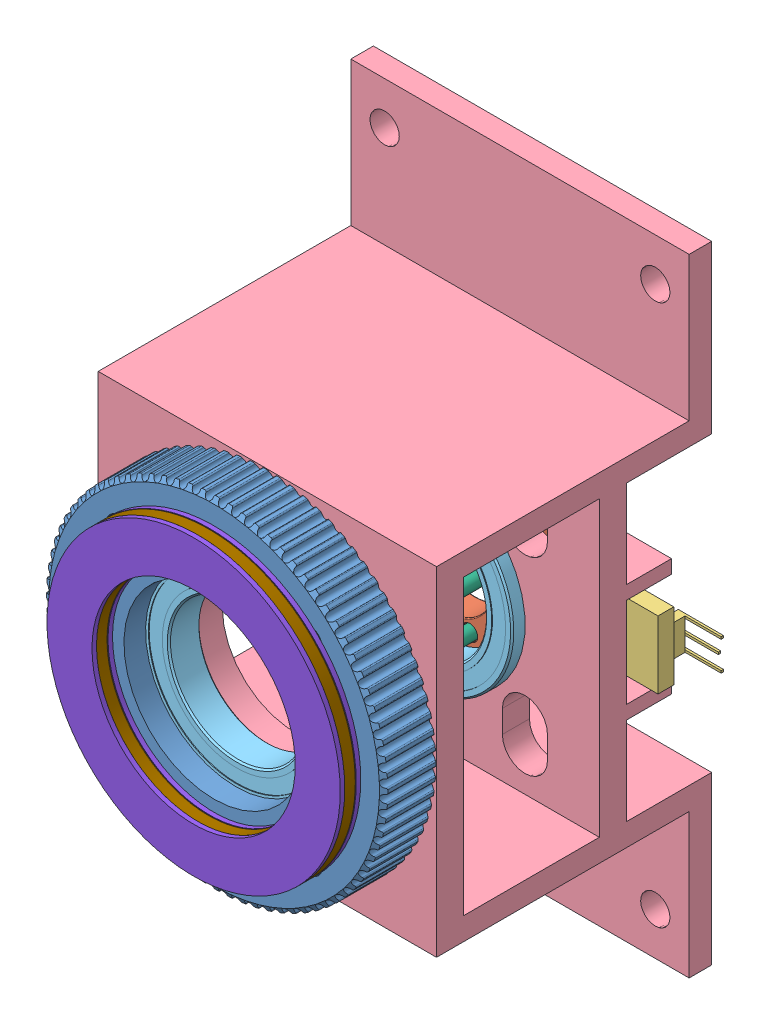
SolidWorks assembly Assem4, configuration Default. Lengths in mm.
Overall size (90.97 138.93 77.35).
21 component instances, 9 part files, 41 mates.
Components (placement in the parent):
- pulleyHTD3m80Tbase-1: pulleyHTD3m80Tbase [Default] at (-84.3677 -23.5327 77.284) x (0 -1 0) z (0 0 -1) size (75.63 75.63 12)
- shaftJ1endPlate-1: shaftJ1endPlate [Default] at (-84.3677 -23.5327 31.3856) x (-0.923728 -0.383049 0) z (0 0 -1) size (40 40 6)
- MagneticSensorV2-1: MagneticSensorV2 [Default] at (-52.8677 -23.5327 22.8856) size (31 15 9)
- base-1: base [Default] at (-84.3677 -23.5327 65.484) size (75 138.93 61)
- bearing6806 30x42x7-5: bearing6806 30x42x7 [5972K282] at (-84.3677 -23.5327 74.809) x (0.923728 0.383049 0) z (0 0 -1) size (42 42 7)
- bearing6806 30x42x7-9: bearing6806 30x42x7 [5972K282] at (-84.3677 -23.5327 34.7106) x (0.923728 0.383049 0) z (0 0 -1) size (42 42 7)
- socket head cap screw_iso-5: socket head cap screw_iso [ISO 4762 M5 x 16 - 16N] at (-105.3677 -44.5327 60.484) x (0 0 1) z (-1 0 0) size (21 8.5 8.5)
- socket head cap screw_iso-6: socket head cap screw_iso [ISO 4762 M5 x 16 - 16N] at (-63.3677 -2.5327 60.484) x (0 0 1) z (-1 0 0) size (21 8.5 8.5)
- socket head cap screw_iso-7: socket head cap screw_iso [ISO 4762 M5 x 16 - 16N] at (-63.3677 -44.5327 60.484) x (0 0 1) z (-1 0 0) size (21 8.5 8.5)
- socket head cap screw_iso-8: socket head cap screw_iso [ISO 4762 M5 x 16 - 16N] at (-105.3677 -2.5327 60.484) x (0 0 1) z (-1 0 0) size (21 8.5 8.5)
- socket head cap screw_iso-14: socket head cap screw_iso [ISO 4762 M3 x 16 - 16N] at (-79.5796 -35.0793 22.3856) x (0 0 1) z (-1 0 0) size (19 5.5 5.5)
- socket head cap screw_iso-15: socket head cap screw_iso [ISO 4762 M3 x 16 - 16N] at (-89.1558 -11.9861 22.3856) x (0 0 1) z (-1 0 0) size (19 5.5 5.5)
- socket head cap screw_iso-16: socket head cap screw_iso [ISO 4762 M3 x 16 - 16N] at (-95.9143 -28.3208 22.3856) x (0 0 1) z (-1 0 0) size (19 5.5 5.5)
- socket head cap screw_iso-17: socket head cap screw_iso [ISO 4762 M3 x 16 - 16N] at (-72.8211 -18.7446 22.3856) x (0 0 1) z (-1 0 0) size (19 5.5 5.5)
- socket head cap screw_iso-19: socket head cap screw_iso [ISO 4762 M2 x 8 - 8N] at (-60.8677 -18.5327 17.3856) x (0 0 1) z (-1 0 0) size (10 3.8 3.8)
- socket head cap screw_iso-20: socket head cap screw_iso [ISO 4762 M2 x 8 - 8N] at (-60.8677 -28.5327 17.3856) x (0 0 1) z (-1 0 0) size (10 3.8 3.8)
- hex thin nut chamfered gradeab_iso-5: hex thin nut chamfered gradeab_iso [ISO - 4035 - M2 - N] at (-60.8677 -28.5327 27.5856) size (4 4.62 1.2)
- hex thin nut chamfered gradeab_iso-6: hex thin nut chamfered gradeab_iso [ISO - 4035 - M2 - N] at (-60.8677 -18.5327 27.5856) size (4 4.62 1.2)
- Washer45x60x1-1: Washer45x60x1 [5909K79] at (-84.3677 -23.5327 87.334) x (0 0 -1) z (1 0 0) size (1 65 65)
- NeedleThrustBearing5909_45x60x3-1: NeedleThrustBearing5909_45x60x3 [5909K19] at (-84.3677 -23.5327 85.559) x (0.923728 0.383049 0) z (-0.383049 0.923728 0) size (65 3 65)
- Washer45x60x1-2: Washer45x60x1 [5909K79] at (-84.3677 -23.5327 83.784) x (0 0 -1) z (1 0 0) size (1 65 65)
Mates (geometry in assembly coordinates):
- Concentric8: concentric aligned: cylinder of pulleyHTD3m80Tbase-1 through (-84.3677 -23.5327 78.484) axis (0 0 -1) radius 21.05; cylinder of base-1 through (-84.3677 -23.5327 71.484) axis (0 0 -1) radius 16
- Coincident14: coincident anti-aligned: plane of pulleyHTD3m80Tbase-1 through (-84.3677 -23.5327 71.484) normal (0 0 -1); plane of base-1 through (-84.3677 -23.5327 71.484) normal (0 0 1)
- Concentric9: concentric aligned: cylinder of pulleyHTD3m80Tbase-1 through (-63.3677 -44.5327 83.284) axis (0 0 -1) radius 3; cylinder of base-1 through (-63.3677 -44.5327 71.484) axis (0 0 -1) radius 2.75
- Concentric10: concentric aligned: cylinder of pulleyHTD3m80Tbase-1 through (-84.3677 -23.5327 83.284) axis (0 0 -1) radius 20; cylinder of bearing6806 30x42x7-5 through (-84.3677 -23.5327 71.309) axis (0 0 -1) radius 21
- Coincident15: coincident anti-aligned: plane of base-1 through (-84.3677 -23.5327 71.484) normal (0 0 1); plane of bearing6806 30x42x7-5 through (-76.8836 -41.5807 71.484) normal (0 0 -1)
- Concentric13: concentric aligned: cylinder of base-1 through (-84.3677 -23.5327 94.924) axis (0 0 -1) radius 21.05; cylinder of bearing6806 30x42x7-9 through (-84.3677 -23.5327 31.2106) axis (0 0 -1) radius 21
- Coincident17: coincident anti-aligned: plane of base-1 through (-84.3677 -23.5327 31.3856) normal (0 0 1); plane of bearing6806 30x42x7-9 through (-76.8836 -41.5807 31.3856) normal (0 0 -1)
- Coincident18: coincident anti-aligned: plane of shaftJ1endPlate-1 through (-84.3677 -23.5327 31.3856) normal (0 0 1); plane of bearing6806 30x42x7-9 through (-76.8836 -41.5807 31.3856) normal (0 0 -1)
- Concentric15: concentric aligned: cylinder of shaftJ1endPlate-1 through (-84.3677 -23.5327 31.3856) axis (0 0 -1) radius 10; cylinder of base-1 through (-84.3677 -23.5327 31.3856) axis (0 0 -1) radius 19.05
- Concentric16: concentric anti-aligned: cylinder of MagneticSensorV2-1 through (-60.8677 -28.5327 27.8856) axis (0 0 -1) radius 1.25; cylinder of base-1 through (-60.8677 -28.5327 19.3856) axis (0 0 1) radius 1.25
- Coincident20: coincident anti-aligned: plane of MagneticSensorV2-1 through (-52.8677 -23.5327 22.8856) normal (0 0 -1); plane of base-1 through (-53.3677 -36.5327 22.8856) normal (0 0 1)
- Concentric21: concentric aligned: cylinder of base-1 through (-105.3677 -44.5327 71.484) axis (0 0 -1) radius 2.75; cylinder of socket head cap screw_iso-5 through (-105.3677 -44.5327 28.734) axis (0 0 -1) radius 4.25
- Coincident25: coincident anti-aligned: plane of base-1 through (-84.3677 -23.5327 65.484) normal (0 0 -1); plane of socket head cap screw_iso-5 through (-105.3677 -40.2827 65.484) normal (0 0 1)
- Concentric22: concentric aligned: cylinder of base-1 through (-63.3677 -2.5327 71.484) axis (0 0 -1) radius 2.75; cylinder of socket head cap screw_iso-6 through (-63.3677 -2.5327 28.734) axis (0 0 -1) radius 4.25
- Coincident26: coincident anti-aligned: plane of base-1 through (-84.3677 -23.5327 65.484) normal (0 0 -1); plane of socket head cap screw_iso-6 through (-63.3677 1.7173 65.484) normal (0 0 1)
- Concentric23: concentric aligned: cylinder of base-1 through (-63.3677 -44.5327 71.484) axis (0 0 -1) radius 2.75; cylinder of socket head cap screw_iso-7 through (-63.3677 -44.5327 28.734) axis (0 0 -1) radius 4.25
- Coincident27: coincident anti-aligned: plane of base-1 through (-84.3677 -23.5327 65.484) normal (0 0 -1); plane of socket head cap screw_iso-7 through (-63.3677 -40.2827 65.484) normal (0 0 1)
- Concentric24: concentric aligned: cylinder of base-1 through (-105.3677 -2.5327 71.484) axis (0 0 -1) radius 2.75; cylinder of socket head cap screw_iso-8 through (-105.3677 -2.5327 28.734) axis (0 0 -1) radius 4.25
- Coincident28: coincident anti-aligned: plane of base-1 through (-84.3677 -23.5327 65.484) normal (0 0 -1); plane of socket head cap screw_iso-8 through (-105.3677 1.7173 65.484) normal (0 0 1)
- Concentric29: concentric anti-aligned: cylinder of shaftJ1endPlate-1 through (-79.5796 -35.0793 25.3856) axis (0 0 1) radius 1.75; cylinder of socket head cap screw_iso-14 through (-79.5796 -35.0793 -9.3644) axis (0 0 -1) radius 2.75
- Coincident33: coincident anti-aligned: plane of shaftJ1endPlate-1 through (-84.3677 -23.5327 25.3856) normal (0 0 -1); plane of socket head cap screw_iso-14 through (-79.5796 -32.3293 25.3856) normal (0 0 1)
- Concentric30: concentric anti-aligned: cylinder of shaftJ1endPlate-1 through (-89.1558 -11.9861 25.3856) axis (0 0 1) radius 1.75; cylinder of socket head cap screw_iso-15 through (-89.1558 -11.9861 -9.3644) axis (0 0 -1) radius 2.75
- Coincident34: coincident anti-aligned: plane of shaftJ1endPlate-1 through (-84.3677 -23.5327 25.3856) normal (0 0 -1); plane of socket head cap screw_iso-15 through (-89.1558 -9.2361 25.3856) normal (0 0 1)
- Concentric31: concentric anti-aligned: cylinder of shaftJ1endPlate-1 through (-95.9143 -28.3208 25.3856) axis (0 0 1) radius 1.75; cylinder of socket head cap screw_iso-16 through (-95.9143 -28.3208 -9.3644) axis (0 0 -1) radius 2.75
- Coincident35: coincident anti-aligned: plane of shaftJ1endPlate-1 through (-84.3677 -23.5327 25.3856) normal (0 0 -1); plane of socket head cap screw_iso-16 through (-95.9143 -25.5708 25.3856) normal (0 0 1)
- Concentric32: concentric anti-aligned: cylinder of shaftJ1endPlate-1 through (-72.8211 -18.7446 25.3856) axis (0 0 1) radius 1.75; cylinder of socket head cap screw_iso-17 through (-72.8211 -18.7446 -9.3644) axis (0 0 -1) radius 2.75
- Coincident36: coincident anti-aligned: plane of shaftJ1endPlate-1 through (-84.3677 -23.5327 25.3856) normal (0 0 -1); plane of socket head cap screw_iso-17 through (-72.8211 -15.9946 25.3856) normal (0 0 1)
- Concentric33: concentric anti-aligned: cylinder of base-1 through (-60.8677 -18.5327 19.3856) axis (0 0 1) radius 1.25; cylinder of socket head cap screw_iso-19 through (-60.8677 -18.5327 -14.3644) axis (0 0 -1) radius 1.9
- Coincident37: coincident anti-aligned: plane of base-1 through (-84.3677 -23.5327 19.3856) normal (0 0 -1); plane of socket head cap screw_iso-19 through (-60.8677 -16.6327 19.3856) normal (0 0 1)
- Concentric34: concentric anti-aligned: cylinder of base-1 through (-60.8677 -28.5327 19.3856) axis (0 0 1) radius 1.25; cylinder of socket head cap screw_iso-20 through (-60.8677 -28.5327 -14.3644) axis (0 0 -1) radius 1.9
- Coincident38: coincident anti-aligned: plane of base-1 through (-84.3677 -23.5327 19.3856) normal (0 0 -1); plane of socket head cap screw_iso-20 through (-60.8677 -26.6327 19.3856) normal (0 0 1)
- Concentric37: concentric anti-aligned: cylinder of MagneticSensorV2-1 through (-60.8677 -28.5327 27.8856) axis (0 0 -1) radius 1.25; cylinder of hex thin nut chamfered gradeab_iso-5 through (-60.8677 -28.5327 2.5481) axis (0 0 1) radius 1
- Coincident41: coincident anti-aligned: plane of MagneticSensorV2-1 through (-52.8677 -23.5327 26.3856) normal (0 0 1); plane of hex thin nut chamfered gradeab_iso-5 through (-60.8677 -26.2233 26.3856) normal (0 0 -1)
- Concentric38: concentric anti-aligned: cylinder of MagneticSensorV2-1 through (-60.8677 -18.5327 27.8856) axis (0 0 -1) radius 1.25; cylinder of hex thin nut chamfered gradeab_iso-6 through (-60.8677 -18.5327 2.5481) axis (0 0 1) radius 1
- Coincident42: coincident anti-aligned: plane of MagneticSensorV2-1 through (-52.8677 -23.5327 26.3856) normal (0 0 1); plane of hex thin nut chamfered gradeab_iso-6 through (-60.8677 -16.2233 26.3856) normal (0 0 -1)
- Coincident43: coincident anti-aligned: plane of pulleyHTD3m80Tbase-1 through (-84.3677 -23.5327 83.284) normal (0 0 1); plane of Washer45x60x1-2 through (-84.3677 -23.5327 83.284) normal (0 0 -1)
- Concentric42: concentric anti-aligned: cylinder of pulleyHTD3m80Tbase-1 through (-84.3677 -23.5327 83.284) axis (0 0 -1) radius 20; cylinder of Washer45x60x1-2 through (-84.3677 -23.5327 83.284) axis (0 0 1) radius 22.525
- Concentric43: concentric aligned: cylinder of pulleyHTD3m80Tbase-1 through (-84.3677 -23.5327 83.284) axis (0 0 -1) radius 20; cylinder of NeedleThrustBearing5909_45x60x3-1 through (-84.3677 -23.5327 84.059) axis (0 0 -1) radius 22.525
- Coincident45: coincident anti-aligned: plane of NeedleThrustBearing5909_45x60x3-1 through (-74.7914 -46.6259 84.284) normal (0 0 -1); plane of Washer45x60x1-2 through (-84.3677 -23.5327 84.284) normal (0 0 1)
- Coincident49: coincident anti-aligned: plane of Washer45x60x1-1 through (-84.3677 -23.5327 86.834) normal (0 0 -1); plane of NeedleThrustBearing5909_45x60x3-1 through (-75.1075 -45.8639 86.834) normal (0 0 1)
- Concentric46: concentric anti-aligned: cylinder of Washer45x60x1-1 through (-84.3677 -23.5327 86.834) axis (0 0 1) radius 22.525; cylinder of NeedleThrustBearing5909_45x60x3-1 through (-84.3677 -23.5327 84.059) axis (0 0 -1) radius 22.525
